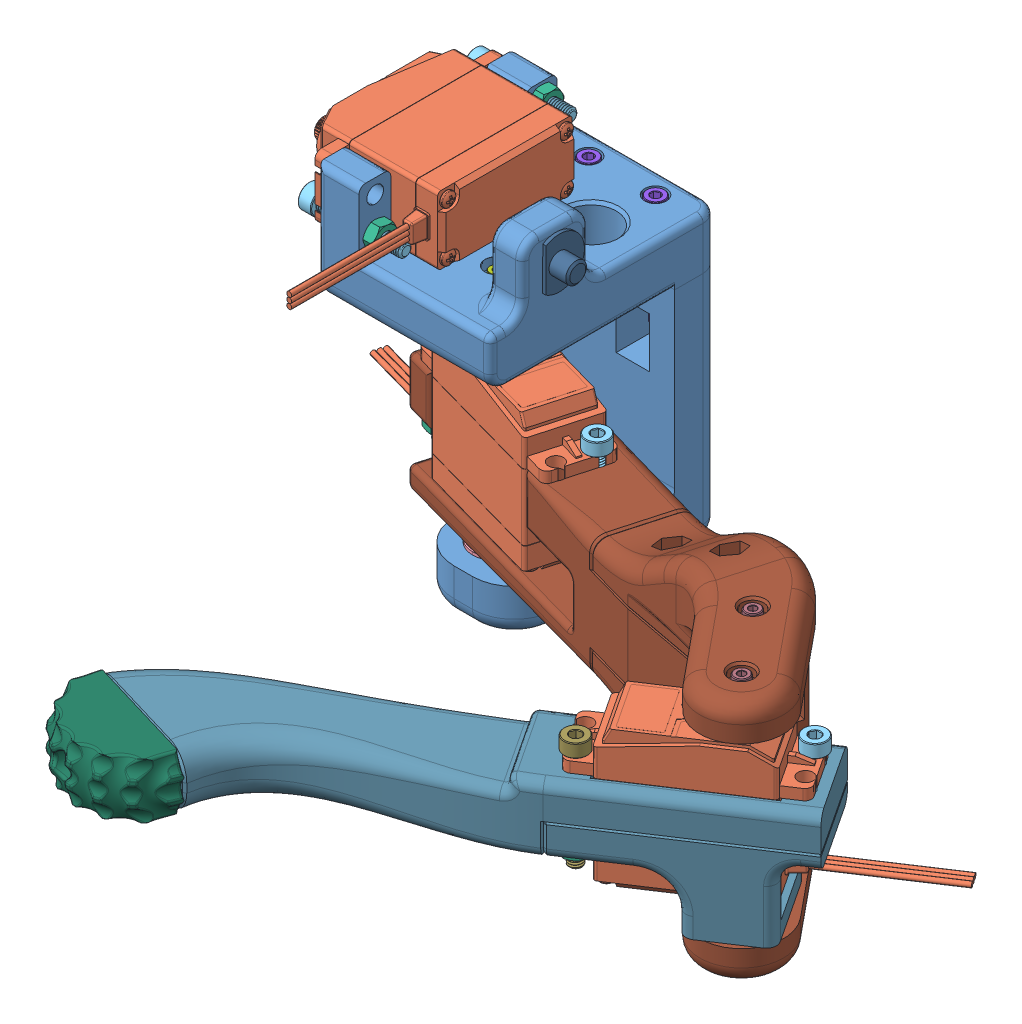
SolidWorks assembly Jambe_droite, configuration Default. Lengths in mm.
Overall size (241.56 105.95 215.04).
41 component instances, 15 part files, 4 mates.
Components (placement in the parent):
- Hanche_V3_D-1: Hanche_V3_D [Default] at origin size (76.1 105.4 99.1)
  - Hanche_V3_D2-1: Hanche_V3_D2 [Default] at origin size (51.8 104.55 68.65)
  - Servo_DS3225MG-1: Servo_DS3225MG [Default] at (-27.6 10.2 0) x (0 0 -1) z (-1 0 0) size (87.25 20.4 45.91)
  - Servo_helice-1: Servo_helice [Défaut] at (24 -10 0) x (-1 0 0) z (0 1 0) size (35.39 15.87 6)
  - bearing_535198-1: bearing_535198 [Défaut] at (24 -75.1322 0) size (13.87 4.75 13.87)
  - M4x25mm-1: M4x25mm [91290A176] at (12 15.2 -34.8) x (0 -0.924225 -0.381849) z (1 0 0) size (7 7 29.41)
  - M4x25mm-2: M4x25mm [91290A176] at (12 5.2 14.8) x (0 -0.924225 -0.381849) z (1 0 0) size (7 7 29.41)
  - M4_nut-1: M4_nut [90592A090] at (4.3 15.2 -34.8) x (0 1 0) z (0 0 1) size (7 3.75 8.08)
  - M4_nut-2: M4_nut [90592A090] at (4.3 5.2 14.8) x (0 0.381849 -0.924225) z (0 -0.924225 -0.381849) size (7 3.75 8.08)
  - M2x16mm-1: M2x16mm [91290A047] at (0 -18.4 0) x (1 0 0) z (0 -1 0) size (3.8 3.8 18.16)
  - M2x16mm-2: M2x16mm [91290A047] at (24 -19 0) x (1 0 0) z (0 -1 0) size (3.8 3.8 18.16)
  - M3x30mm-1: M3x30mm [91290A171] at (9.5 -33 -42.25) x (1 0 0) z (0 -1 0) size (5.5 5.5 33.33)
  - M3x30mm-2: M3x30mm [91290A171] at (29.5 -33 -42.25) x (1 0 0) z (0 -1 0) size (5.5 5.5 33.33)
  - M3_nut-1: M3_nut [90592A085] at (29.5 -26.2 -42.25) size (5.5 2.79 6.35)
  - M3_nut-2: M3_nut [90592A085] at (9.5 -26.2 -42.25) size (5.5 2.79 6.35)
  - Cylinde_bearing-1: Cylinde_bearing [Default] at (24 -75.8824 0) x (0.999973 0 0.007405) z (0 1 0) size (15 11.5 12)
  - Cylinde_bearing-2: Cylinde_bearing [Default] at (36.5 10.2 0) x (0 -0.999973 0.007405) z (1 0 0) size (15 11.5 12)
- Femur_D-1: Femur_D [Default] at (24 -49.05 0) x (0 1 0) z (0.962961 0 0.269641) size (73 46.33 202.15)
  - Femur_V3_D-1: Femur_V3_D [Default] at origin size (73 46.33 172.05)
  - Servo_DS3225MG-1: Servo_DS3225MG [Default] at (36.05 0 0) x (0 0 1) z (1 0 0) size (87.25 20.4 45.91)
  - M4x25mm-1: M4x25mm [91290A176] at (-3.55 5 -14.8) x (0 0.921619 0.388095) z (-1 0 0) size (7 7 29.41)
  - M4x25mm-2: M4x25mm [91290A176] at (-3.55 -5 34.8) x (0 0.921619 0.388095) z (-1 0 0) size (7 7 29.41)
  - M4_nut-1: M4_nut [90592A090] at (1.65 -5 34.8) x (0 -1 0) z (0 0 1) size (7 3.75 8.08)
  - M4_nut-2: M4_nut [90592A090] at (1.65 5 -14.8) x (0 -1 0) z (0 0 1) size (7 3.75 8.08)
  - M4x30mm-1: M4x30mm [91290A180] at (17 -2.3 71.7972) x (0 0 -1) z (1 0 0) size (7 7 34.38)
  - M4x30mm-2: M4x30mm [91290A180] at (17 -2.3 96.7972) x (0 0 -1) z (1 0 0) size (7 7 34.38)
  - M4_nut-3: M4_nut [90592A090] at (14.6 -2.3 71.7972) x (0 0.5 -0.866025) z (0 -0.866025 -0.5) size (7 3.75 8.08)
  - M4_nut-4: M4_nut [90592A090] at (14.6 -2.3 96.7972) x (0 -1 0) z (0 0 -1) size (7 3.75 8.08)
  - Servo_helice-1: Servo_helice [Défaut] at (32.5 18.86 139.55) x (0 -0.573576 -0.819152) z (1 0 0) size (35.39 15.87 6)
  - M2_8-1: M2_8 [91292A012] at (25.5 18.86 139.55) x (0 0 1) z (-1 0 0) size (4.5 4.5 10.65)
  - M2_8-2: M2_8 [91292A012] at (25.5 5.0942 119.8904) x (0 0 1) z (-1 0 0) size (4.5 4.5 10.65)
- Tibia_D-1: Tibia_D [Default] at (153.2958 -37.4324 55.7898) x (-0.83474 0 0.550644) z (0.550644 0 0.83474) size (207.93 61.42 52.63)
  - Tibia_V3_D-1: Tibia_V3_D [Default] at origin size (162.76 36.13 39.97)
  - Embout_TPE_V3-1: Embout_TPE_V3 [Default] at (129.9518 11.7 0.0575) x (0 -1 0) z (0.642788 0 -0.766044) size (17.12 19.75 39.79)
  - Servo_DS3225MG-1: Servo_DS3225MG [Default] at (0 -17.8 0) x (1 0 0) z (0 -1 0) size (87.25 20.4 45.91)
  - bearing_535198-1: bearing_535198 [Défaut] at (0 32.3678 0) size (13.87 4.75 13.87)
  - Cylinde_bearing-1: Cylinde_bearing [Default] at (0 31.6176 0) x (0 0 -1) z (0 1 0) size (15 11.5 12)
  - M4x25mm-1: M4x25mm [91290A176] at (-14.8 21.8 -5) x (1 0 0) z (0 1 0) size (7 7 29.41)
  - M4x30mm-1: M4x30mm [91290A180] at (34.8 26.8 5) x (-0.986333 0 -0.164763) z (0 1 0) size (7 7 34.38)
  - M4_nut-1: M4_nut [90592A090] at (34.8 21.6 5) x (0.873041 0 -0.487647) z (0.487647 0 0.873041) size (7 3.75 8.08)
  - M4_nut-2: M4_nut [90592A090] at (-14.8 16.6 -5) x (0.873041 0 -0.487647) z (0.487647 0 0.873041) size (7 3.75 8.08)
Mates (geometry in assembly coordinates):
- Concentric2: concentric anti-aligned: cylinder of Hanche_V3_D-1/Cylinde_bearing-1 through (24 -63.8824 0) axis (0 -1 0) radius 3.1; cylinder of Femur_D-1/Femur_V3_D-1 through (24 -59.8 0) axis (0 1 0) radius 3.15
- Concentric4: concentric aligned: cylinder of Femur_D-1/Femur_V3_D-1 through (153.2958 -83.05 55.7898) axis (0 1 0) radius 3.15; cylinder of Tibia_D-1/Cylinde_bearing-1 through (153.2958 -81.05 55.7898) axis (0 1 0) radius 3.1
- Coincident3: coincident anti-aligned: plane of Femur_D-1/Femur_V3_D-1 through (135.9271 -75.55 164.1761) normal (0 1 0); plane of Tibia_D-1/Cylinde_bearing-1 through (153.2958 -75.55 55.7898) normal (0 -1 0)
- Coincident4: coincident anti-aligned: plane of Hanche_V3_D-1/Servo_helice-1 through (24 -13 0) normal (0 -1 0); plane of Femur_D-1/Servo_DS3225MG-1 through (24 -13 0) normal (0 1 0)
